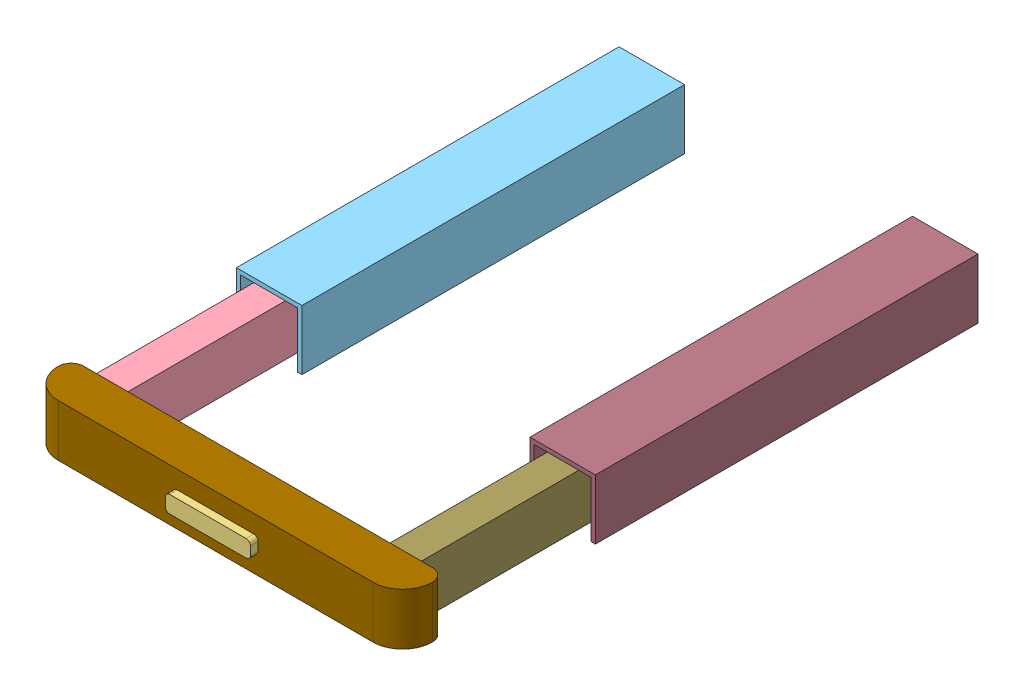
SolidWorks assembly LaGan, configuration 默认. Lengths in mm.
Overall size (440 70.5 694.69).
24 component instances, 22 part files, 0 mates.
Components (placement in the parent):
- LaGan.stp-1: LaGan.stp [默认] at origin size (440 70.5 694.69)
  - Part1.stp-1: Part1.stp [默认] at (-5.6752 0 -212.5) size (15 50 35)
  - Part2.stp-1: Part2.stp [默认] at (-6.3813 0 -177.2239) size (27 50 70)
  - Symmetry of Part1.stp-1: Symmetry of Part1.stp [默认] at (-7.1999 0 -212.5) x (-1 0 0) z (0 0 1) size (15 50 35)
  - Part3.stp-1: Part3.stp [默认] at (-6.3813 0 0) size (37 60 585.6)
  - Part4.stp-1: Part4.stp [默认] at (-6.3813 0 0) size (77 70.5 450)
  - Part6.stp-1: Part6.stp [默认] at (-6.3813 1.8634 -149.7239) x (0 -1 0) z (0 0 1) size (53 8 8)
  - Part7.stp-1: Part7.stp [默认] at (-14.4565 -13.3194 -224.6748) x (0 0 -1) z (1 0 0) size (5.87 5.79 19.66)
  - Part8.stp-1: Part8.stp [默认] at (-14.4565 11.5233 -224.6748) x (0 0 -1) z (1 0 0) size (5.87 5.79 19.66)
  - Part9.stp-1: Part9.stp [默认] at (166.1925 0 0) size (440 61 50)
  - Symmetry of Part1.stp-2: Symmetry of Part1.stp [默认] at (338.0603 0 -212.5) x (-1 0 0) z (0 0 1) size (15 50 35)
  - Symmetry of Part2.stp-1: Symmetry of Part2.stp [默认] at (338.7664 0 -177.2239) x (-1 0 0) z (0 0 1) size (27 50 70)
  - Symmetry of Symmetry of Part1.stp-1: Symmetry of Symmetry of Part1.stp [默认] at (339.5849 0 -212.5) size (15 50 35)
  - Symmetry of Part3.stp-1: Symmetry of Part3.stp [默认] at (338.7664 0 0) x (-1 0 0) z (0 0 1) size (37 60 585.6)
  - Symmetry of Part4.stp-1: Symmetry of Part4.stp [默认] at (338.7664 0 0) x (-1 0 0) z (0 0 1) size (77 70.5 450)
  - Symmetry of Part5.stp-1: Symmetry of Part5.stp [默认] at (338.7664 0 -149.7239) x (-1 0 0) z (0 0 1) size (21 21 533)
  - Symmetry of Part6.stp-1: Symmetry of Part6.stp [默认] at (338.7664 1.8634 -149.7239) x (0 -1 0) z (0 0 1) size (53 8 8)
  - Symmetry of Part8.stp-1: Symmetry of Part8.stp [默认] at (346.8416 11.5233 -224.6748) x (0 0 -1) z (-1 0 0) size (5.87 5.79 19.66)
  - Symmetry of Part7.stp-1: Symmetry of Part7.stp [默认] at (346.8416 -13.3194 -224.6748) x (0 0 -1) z (-1 0 0) size (5.87 5.79 19.66)
  - Part10.stp-1: Part10.stp [默认] at (266.1925 0 364.6037) size (160.03 10.01 15)
  - Symmetry of Symmetry of Part5.stp-1: Symmetry of Symmetry of Part5.stp [默认] at (-6.3813 0 -149.7239) size (21 21 533)
  - Symmetry of Part10.stp-1: Symmetry of Part10.stp [默认] at (66.1925 0 364.6037) x (-1 0 0) z (0 0 1) size (160.03 10.01 15)
  - Part11.stp-1: Part11.stp [默认] at (166.1925 0 373.6899) size (100 20 21)
  - Part12.stp-1: Part12.stp [默认] at (166.1925 0 336.6037) size (16.79 17.27 58.78)
